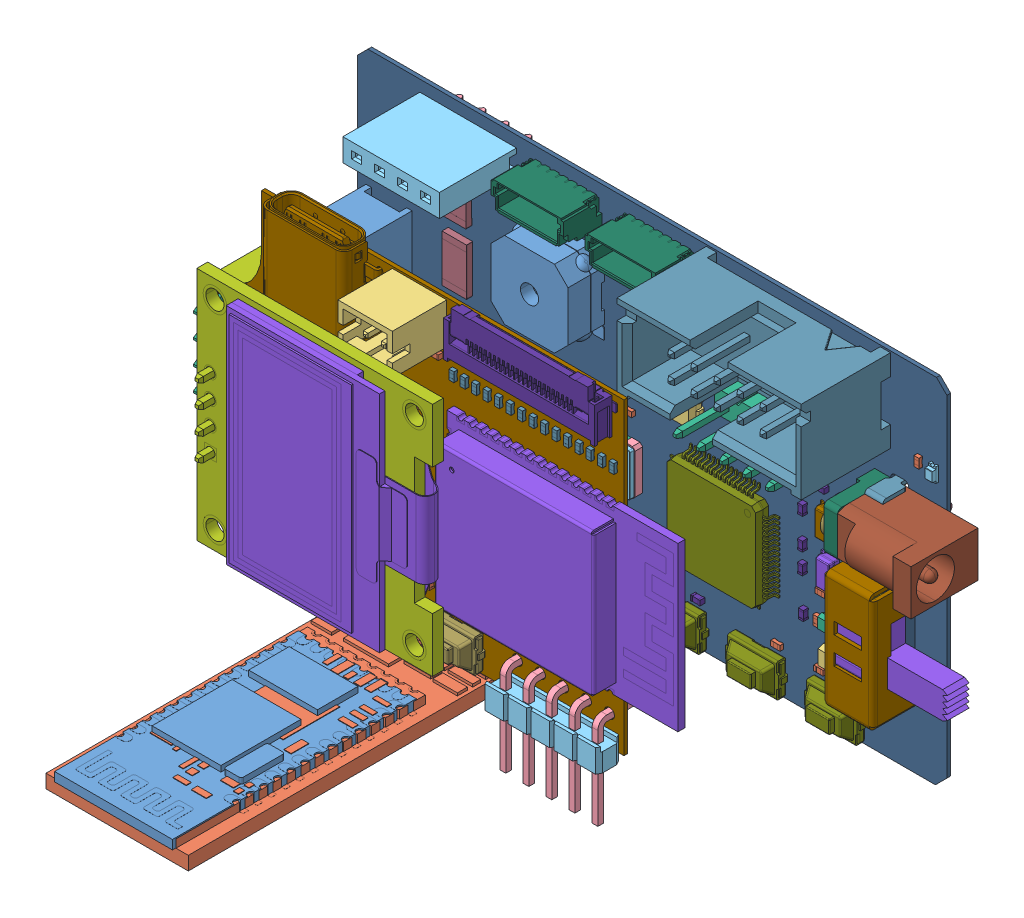
SolidWorks assembly balancing_robot_board, configuration Default. Lengths in mm.
Overall size (69.07 43.84 49.2).
373 component instances, 64 part files, 0 mates.
Components (placement in the parent):
- balancing_robot_board.step-1: balancing_robot_board.step [Default] at origin size (69.07 43.84 49.2)
  - LS.step-1: LS.step [Default] at origin size (8.5 8.5 4.05)
    - KSSG74B17-3--3DModel-STEP-532303.step-1: KSSG74B17-3--3DModel-STEP-532303.step [Default] at (18.4151 23.5629 3.048) x (0 1 0) z (1 0 0) size (8.5 4.05 8.5)
  - R23.step-1: R23.step [Default] at origin size (1.05 0.55 0.4)
    - RES_0402_(1005_metric).step-1: RES_0402_(1005_metric).step [Default] at (30.8864 22.1487 -0.4115) x (1 0 0) z (0 0 -1) size (1.05 0.55 0.4)
  - R21.step-1: R21.step [Default] at origin size (1.05 0.55 0.4)
    - RES_0402_(1005_metric).step-1: RES_0402_(1005_metric).step [Default] at (30.8864 25.3491 -0.4115) x (1 0 0) z (0 0 -1) size (1.05 0.55 0.4)
  - R22.step-1: R22.step [Default] at origin size (1.05 0.55 0.4)
    - RES_0402_(1005_metric).step-1: RES_0402_(1005_metric).step [Default] at (30.8864 23.7489 -0.4115) x (1 0 0) z (0 0 -1) size (1.05 0.55 0.4)
  - D5.step-1: D5.step [Default] at origin size (1.6 0.8 0.7)
    - 6715996480.step-1: 6715996480.step [Default] at (6.731 0.5588 0) x (1 0 0) z (0 -1 0) size (1.6 0.7 0.8)
  - D4.step-1: D4.step [Default] at origin size (1.6 0.8 0.7)
    - 6715996096.step-1: 6715996096.step [Default] at (46.7106 21.463 0) x (1 0 0) z (0 -1 0) size (1.6 0.7 0.8)
  - D3.step-1: D3.step [Default] at origin size (0.8 1.6 0.7)
    - 6715995904.step-1: 6715995904.step [Default] at (63.3476 29.1846 0) x (0 1 0) z (1 0 0) size (1.6 0.7 0.8)
  - Q1.step-1: Q1.step [Default] at origin size (2.92 2.37 1.12)
    - 6715995712.step-1: 6715995712.step [Default] at (52.8829 9.3981 0) x (0 1 0) z (1 0 0) size (2.37 1.12 2.92)
  - S1.step-1: S1.step [Default] at origin size (12.2 13 8.6)
    - User_Library-Assem1-20.step-1: User_Library-Assem1-20.step [Default] at (41.4801 49.8595 5.0375) x (0 1 0) z (1 0 0) size (13 8.6 12.2)
      - User_Library-Assem1-20_Part1.step-1: User_Library-Assem1-20_Part1.step [Default] at (-40.4363 -8.049 18.1299) size (1.5 6.6 0.5)
      - User_Library-Assem1-20_Part3.step-1: User_Library-Assem1-20_Part3.step [Default] at (-40.0863 -3.449 20.2299) size (9 3.9 11.7)
      - User_Library-Assem1-20_Part2.step-1: User_Library-Assem1-20_Part2.step [Default] at (-43.1863 0.551 15.4299) size (13 6 5.6)
      - User_Library-Assem1-20_Part1.step-2: User_Library-Assem1-20_Part1.step [Default] at (-37.4363 -8.049 18.1299) size (1.5 6.6 0.5)
      - User_Library-Assem1-20_Part1.step-3: User_Library-Assem1-20_Part1.step [Default] at (-34.4363 -8.049 18.1299) size (1.5 6.6 0.5)
      - User_Library-Assem1-20_Part4.step-1: User_Library-Assem1-20_Part4.step [Default] at (-30.9863 -4.449 15.5299) size (12.2 1 4.7)
  - ON_OFF.step-1: ON_OFF.step [Default] at origin size (11.6 5.4 10.6)
    - PJ-031D.step-1: PJ-031D.step [Default] at (68.0973 23.6729 0) x (0 1 0) z (1 0 0) size (5 7.4 9.5)
    - PJ-031D-0.step-1: PJ-031D-0.step [Default] at (68.0973 23.6729 0) x (0 1 0) z (1 0 0) size (3 9.2 0.6)
    - PJ-031D-1.step-1: PJ-031D-1.step [Default] at (68.0973 23.6729 0) x (0 1 0) z (1 0 0) size (1 3.2 0.3)
    - PJ-031D-2.step-1: PJ-031D-2.step [Default] at (68.0973 23.6729 0) x (0 1 0) z (1 0 0) size (0.4 6.2 2)
    - PJ-031D-3.step-1: PJ-031D-3.step [Default] at (68.0973 23.6729 0) x (0 1 0) z (1 0 0) size (5 6 1.9)
  - RESET.step-1: RESET.step [Default] at origin size (6.1 3.7 2.5)
    - User_Library-Button-SMD.step-1: User_Library-Button-SMD.step [Default] at (35.4637 1.3971 0) x (1 0 0) z (0 -1 0) size (6.1 2.5 3.7)
  - R14.step-1: R14.step [Default] at origin size (1.05 0.55 0.4)
    - RES_0402_(1005_metric).step-1: RES_0402_(1005_metric).step [Default] at (33.5534 4.1911 0) x (1 0 0) z (0 0 1) size (1.05 0.55 0.4)
  - C20.step-1: C20.step [Default] at origin size (1.05 0.55 0.55)
    - CAP_0402_(1005_metric).step-1: CAP_0402_(1005_metric).step [Default] at (37.4396 4.1909 0) x (-1 0 0) z (0 0 1) size (1.05 0.55 0.55)
  - C19.step-1: C19.step [Default] at origin size (5.08 10.66 11.6)
    - 61300821821.step-1: 61300821821.step [Default] at (3.1241 19.9389 4.26) x (0 1 0) z (0 0 1) size (10.66 5.08 11.6)
      - 6130xx21821_PIN.step-1: 6130xx21821_PIN.step [Default] at (-3.81 -1.47 -3.3268) size (2 0.4 10.2)
      - 6130xx21821_PIN.step-2: 6130xx21821_PIN.step [Default] at (-3.81 1.07 -3.3268) size (2 0.4 10.2)
      - 6130xx21821_PIN.step-3: 6130xx21821_PIN.step [Default] at (-1.27 -1.47 -3.3268) size (2 0.4 10.2)
      - 6130xx21821_PIN.step-4: 6130xx21821_PIN.step [Default] at (-1.27 1.07 -3.3268) size (2 0.4 10.2)
      - 6130xx21821_PIN.step-5: 6130xx21821_PIN.step [Default] at (1.27 -1.47 -3.3268) size (2 0.4 10.2)
      - 6130xx21821_PIN.step-6: 6130xx21821_PIN.step [Default] at (1.27 1.07 -3.3268) size (2 0.4 10.2)
      - 6130xx21821_PIN.step-7: 6130xx21821_PIN.step [Default] at (3.81 -1.47 -3.3268) size (2 0.4 10.2)
      - 6130xx21821_PIN.step-8: 6130xx21821_PIN.step [Default] at (3.81 1.07 -3.3268) size (2 0.4 10.2)
      - 61300821821-4.step-1: 61300821821-4.step [Default] at origin size (10.66 5.08 8.5)
  - STA.TR4.step-1: STA.TR4.step [Default] at origin size (1.4 3 1.14)
    - 6813825728.step-1: 6813825728.step [Default] at (25.1206 29.2354 -1.5515) size (1.4 3 1.14)
      - Extruded.step-1: Extruded.step [Default] at origin size (1.4 3 1.14)
  - STA.TR2.step-1: STA.TR2.step [Default] at origin size (1.4 3 1.14)
    - 6813825728.step-1: 6813825728.step [Default] at (29.9466 29.2354 -1.5515) size (1.4 3 1.14)
      - Extruded.step-1: Extruded.step [Default] at origin size (1.4 3 1.14)
  - STA.TR1.step-1: STA.TR1.step [Default] at origin size (1.4 3 1.14)
    - 6813825728.step-1: 6813825728.step [Default] at (34.798 29.2354 -1.5515) size (1.4 3 1.14)
      - Extruded.step-1: Extruded.step [Default] at origin size (1.4 3 1.14)
  - R28.step-1: R28.step [Default] at origin size (0.55 1.05 0.4)
    - RES_0402_(1005_metric).step-1: RES_0402_(1005_metric).step [Default] at (27.5589 29.6926 -0.4115) x (0 -1 0) z (0 0 -1) size (1.05 0.55 0.4)
  - R27.step-1: R27.step [Default] at origin size (0.55 1.05 0.4)
    - RES_0402_(1005_metric).step-1: RES_0402_(1005_metric).step [Default] at (32.3595 29.6926 -0.4115) x (0 -1 0) z (0 0 -1) size (1.05 0.55 0.4)
  - R24.step-1: R24.step [Default] at origin size (0.55 1.05 0.4)
    - RES_0402_(1005_metric).step-1: RES_0402_(1005_metric).step [Default] at (37.1855 29.6926 -0.4115) x (0 -1 0) z (0 0 -1) size (1.05 0.55 0.4)
  - R20.step-1: R20.step [Default] at origin size (1.05 0.55 0.4)
    - RES_0402_(1005_metric).step-1: RES_0402_(1005_metric).step [Default] at (46.1344 4.1401 0) x (-1 0 0) z (0 0 1) size (1.05 0.55 0.4)
  - R19.step-1: R19.step [Default] at origin size (1.05 0.55 0.4)
    - RES_0402_(1005_metric).step-1: RES_0402_(1005_metric).step [Default] at (50.8762 4.1403 0) x (1 0 0) z (0 0 1) size (1.05 0.55 0.4)
  - D2.step-1: D2.step [Default] at origin size (5.4 5 1.6)
    - 6715994176.step-1: 6715994176.step [Default] at (35.2806 23.749 0) x (1 0 0) z (0 -1 0) size (5.4 1.6 5)
  - CT1.step-1: CT1.step [Default] at origin size (3.2 5 1.3)
    - User_Library-ABM3-1.step-1: User_Library-ABM3-1.step [Default] at (29.5014 13.2335 0) x (0 1 0) z (0 0 1) size (5 3.2 1.3)
      - User_Library-ABM3-1_Fillet002.step-1: User_Library-ABM3-1_Fillet002.step [Default] at origin size (5 3.2 0.85)
      - User_Library-ABM3-1_Fillet001.step-1: User_Library-ABM3-1_Fillet001.step [Default] at (0 0 0.85) size (4.7 2.97 0.45)
      - User_Library-ABM3-1_Pad001.step-1: User_Library-ABM3-1_Pad001.step [Default] at origin size (4.9 2 0.4)
  - C18.step-1: C18.step [Default] at origin size (0.55 1.05 0.55)
    - CAP_0402_(1005_metric).step-1: CAP_0402_(1005_metric).step [Default] at (26.5297 10.9474 0) x (0 -1 0) z (0 0 1) size (1.05 0.55 0.55)
  - C17.step-1: C17.step [Default] at origin size (0.55 1.05 0.55)
    - CAP_0402_(1005_metric).step-1: CAP_0402_(1005_metric).step [Default] at (26.5295 15.494 0) x (0 1 0) z (0 0 1) size (1.05 0.55 0.55)
  - U5.step-1: U5.step [Default] at origin size (3 3 1.05)
    - 6715990144.step-1: 6715990144.step [Default] at (18.3896 16.1544 0) x (1 0 0) z (0 -1 0) size (3 1.05 3)
  - U4.step-1: U4.step [Default] at origin size (2.8 2.9 1.45)
    - 6715990912.step-1: 6715990912.step [Default] at (52.3494 14.4526 0) x (-1 0 0) z (0 1 0) size (2.8 1.45 2.9)
  - U3.step-1: U3.step [Default] at origin size (2.8 2.9 1.45)
    - 6715993792.step-1: 6715993792.step [Default] at (52.2478 19.1262 0) x (-1 0 0) z (0 1 0) size (2.8 1.45 2.9)
  - U2.step-1: U2.step [Default] at origin size (7 6.5 1.8)
    - 6715989760.step-1: 6715989760.step [Default] at (20.193 6.8072 0) x (1 0 0) z (0 -1 0) size (7 1.8 6.5)
  - U1.step-1: U1.step [Default] at origin size (3 3 1)
    - 6715991872.step-1: 6715991872.step [Default] at (4.8768 9.2964 0) x (-1 0 0) z (0 1 0) size (3 1 3)
  - SW2.step-1: SW2.step [Default] at origin size (6.1 3.7 2.5)
    - User_Library-Button-SMD.step-1: User_Library-Button-SMD.step [Default] at (44.1707 1.3971 0) x (1 0 0) z (0 -1 0) size (6.1 2.5 3.7)
  - SW1.step-1: SW1.step [Default] at origin size (6.1 3.7 2.5)
    - User_Library-Button-SMD.step-1: User_Library-Button-SMD.step [Default] at (52.8573 1.3969 0) x (-1 0 0) z (0 1 0) size (6.1 2.5 3.7)
  - STA.TR3.step-1: STA.TR3.step [Default] at origin size (1.4 3 1.14)
    - 6813825728.step-1: 6813825728.step [Default] at (19.7358 29.2354 -1.5515) size (1.4 3 1.14)
      - Extruded.step-1: Extruded.step [Default] at origin size (1.4 3 1.14)
  - R26.step-1: R26.step [Default] at origin size (0.55 1.05 0.4)
    - RES_0402_(1005_metric).step-1: RES_0402_(1005_metric).step [Default] at (22.5297 29.6926 -0.4115) x (0 -1 0) z (0 0 -1) size (1.05 0.55 0.4)
  - R25.step-1: R25.step [Default] at origin size (1.35 2.2 0.7)
    - RES_0805_(2012_metric).step-1: RES_0805_(2012_metric).step [Default] at (16.3323 24.5617 -0.013) x (0 -1 0) z (0 0 1) size (2.2 1.35 0.7)
  - R18.step-1: R18.step [Default] at origin size (0.55 1.05 0.4)
    - RES_0402_(1005_metric).step-1: RES_0402_(1005_metric).step [Default] at (61.6965 29.4466 0) x (0 1 0) z (0 0 1) size (1.05 0.55 0.4)
  - R17.step-1: R17.step [Default] at origin size (0.55 1.05 0.4)
    - RES_0402_(1005_metric).step-1: RES_0402_(1005_metric).step [Default] at (9.2455 0.5588 0) x (0 1 0) z (0 0 1) size (1.05 0.55 0.4)
  - R16.step-1: R16.step [Default] at origin size (0.55 1.05 0.4)
    - RES_0402_(1005_metric).step-1: RES_0402_(1005_metric).step [Default] at (48.9965 21.0646 0) x (0 1 0) z (0 0 1) size (1.05 0.55 0.4)
  - R15.step-1: R15.step [Default] at origin size (1.05 0.55 0.4)
    - RES_0402_(1005_metric).step-1: RES_0402_(1005_metric).step [Default] at (29.7608 18.2625 0) x (-1 0 0) z (0 0 1) size (1.05 0.55 0.4)
  - R13.step-1: R13.step [Default] at origin size (0.55 1.05 0.4)
    - RES_0402_(1005_metric).step-1: RES_0402_(1005_metric).step [Default] at (1.2315 7.8282 0) x (0 1 0) z (0 0 1) size (1.05 0.55 0.4)
  - R12.step-1: R12.step [Default] at origin size (0.55 1.05 0.4)
    - RES_0402_(1005_metric).step-1: RES_0402_(1005_metric).step [Default] at (1.2823 10.3094 0) x (0 1 0) z (0 0 1) size (1.05 0.55 0.4)
  - R11.step-1: R11.step [Default] at origin size (1.05 0.55 0.4)
    - RES_0402_(1005_metric).step-1: RES_0402_(1005_metric).step [Default] at (1.7316 5.5087 0) x (-1 0 0) z (0 0 1) size (1.05 0.55 0.4)
  - R10.step-1: R10.step [Default] at origin size (1.05 0.55 0.4)
    - RES_0402_(1005_metric).step-1: RES_0402_(1005_metric).step [Default] at (5.8544 12.8495 0) x (1 0 0) z (0 0 1) size (1.05 0.55 0.4)
  - R9.step-1: R9.step [Default] at origin size (0.55 1.05 0.4)
    - RES_0402_(1005_metric).step-1: RES_0402_(1005_metric).step [Default] at (8.2927 8.0742 0) x (0 1 0) z (0 0 1) size (1.05 0.55 0.4)
  - R8.step-1: R8.step [Default] at origin size (0.55 1.05 0.4)
    - RES_0402_(1005_metric).step-1: RES_0402_(1005_metric).step [Default] at (8.2675 10.4364 0) x (0 -1 0) z (0 0 1) size (1.05 0.55 0.4)
  - R7.step-1: R7.step [Default] at origin size (2.7 5.2 0.7)
    - RES_2010_(5025_metric).step-1: RES_2010_(5025_metric).step [Default] at (10.9221 29.7687 -0.013) x (0 -1 0) z (0 0 1) size (5.2 2.7 0.7)
  - R6.step-1: R6.step [Default] at origin size (2.7 5.2 0.7)
    - RES_2010_(5025_metric).step-1: RES_2010_(5025_metric).step [Default] at (10.9981 23.0773 -0.013) x (0 1 0) z (0 0 1) size (5.2 2.7 0.7)
  - R5.step-1: R5.step [Default] at origin size (0.55 1.05 0.4)
    - RES_0402_(1005_metric).step-1: RES_0402_(1005_metric).step [Default] at (13.8939 7.239 0) x (0 -1 0) z (0 0 1) size (1.05 0.55 0.4)
  - R4.step-1: R4.step [Default] at origin size (0.55 1.05 0.4)
    - RES_0402_(1005_metric).step-1: RES_0402_(1005_metric).step [Default] at (13.8939 4.9276 0) x (0 -1 0) z (0 0 1) size (1.05 0.55 0.4)
  - R3.step-1: R3.step [Default] at origin size (1.05 0.55 0.4)
    - RES_0402_(1005_metric).step-1: RES_0402_(1005_metric).step [Default] at (51.0286 11.6333 0) x (1 0 0) z (0 0 1) size (1.05 0.55 0.4)
  - R2.step-1: R2.step [Default] at origin size (1.05 0.55 0.4)
    - RES_0402_(1005_metric).step-1: RES_0402_(1005_metric).step [Default] at (54.8386 11.6333 0) x (1 0 0) z (0 0 1) size (1.05 0.55 0.4)
  - R1.step-1: R1.step [Default] at origin size (0.55 1.05 0.4)
    - RES_0402_(1005_metric).step-1: RES_0402_(1005_metric).step [Default] at (50.5461 8.6948 0) x (0 -1 0) z (0 0 1) size (1.05 0.55 0.4)
  - P1.step-1: P1.step [Default] at origin size (20.32 9.14 12.9)
    - User_Library-Tyco_-_5103308-1_(Shrouded_Header_2_54mm_10_Pin).step-1: User_Library-Tyco_-_5103308-1_(Shrouded_Header_2_54mm_10_Pin).step [Default] at (48.2856 33.5278 0) x (1 0 0) z (0 -1 0) size (20.32 12.9 9.14)
  - J4.step-1: J4.step [Default] at origin size (8 3.6 4.25)
    - 6715990528.step-1: 6715990528.step [Default] at (22.606 36.2966 0) x (1 0 0) z (0 -1 0) size (8 4.25 3.6)
      - BMxxB-SRSS-TB(LF)(SN)_06.step-1: BMxxB-SRSS-TB(LF)(SN)_06.step [Default] at (0 0 0.75) size (8 4.25 3.6)
  - J3.step-1: J3.step [Default] at origin size (8 3.6 4.25)
    - 6715990528.step-1: 6715990528.step [Default] at (32.9932 36.2682 0) x (1 0 0) z (0 -1 0) size (8 4.25 3.6)
      - BMxxB-SRSS-TB(LF)(SN)_06.step-1: BMxxB-SRSS-TB(LF)(SN)_06.step [Default] at (0 0 0.75) size (8 4.25 3.6)
  - J1.step-1: J1.step [Default] at origin size (12 12 1.6)
    - 6715993024.step-1: 6715993024.step [Default] at (40.259 12.4714 0) x (0 -1 0) z (-1 0 0) size (12 1.6 12)
  - HC1.step-1: HC1.step [Default] at origin size (15.74 7.73 49.09)
    - 61300611821.step-1: 61300611821.step [Default] at (18.7197 0.9143 4.26) x (-1 0 0) z (0 0 1) size (15.74 2.5 11.6)
      - 6130xx11821_PIN.step-1: 6130xx11821_PIN.step [Default] at (-6.35 -0.2 -3.3268) size (2 0.4 10.2)
      - 6130xx11821_PIN.step-2: 6130xx11821_PIN.step [Default] at (-3.81 -0.2 -3.3268) size (2 0.4 10.2)
      - 6130xx11821_PIN.step-3: 6130xx11821_PIN.step [Default] at (-1.27 -0.2 -3.3268) size (2 0.4 10.2)
      - 6130xx11821_PIN.step-4: 6130xx11821_PIN.step [Default] at (1.27 -0.2 -3.3268) size (2 0.4 10.2)
      - 6130xx11821_PIN.step-5: 6130xx11821_PIN.step [Default] at (3.81 -0.2 -3.3268) size (2 0.4 10.2)
      - 6130xx11821_PIN.step-6: 6130xx11821_PIN.step [Default] at (6.35 -0.2 -3.3268) size (2 0.4 10.2)
      - 61300611821-5.step-1: 61300611821-5.step [Default] at origin size (15.74 2.5 8.5)
    - HC-06.step-1: HC-06.step [Default] at (25.2198 -3.0227 46) x (0 0 -1) z (1 0 0) size (26.9 1.63 13)
    - Bluetooth_4.0_BLE.step-1: Bluetooth_4.0_BLE.step [Default] at (18.7199 -3.0627 8) x (0 0 1) z (-1 0 0) size (44.38 6.8 15.7)
  - D1.step-1: D1.step [Default] at origin size (3.9 1.8 1.18)
    - SOD123.step-1: SOD123.step [Default] at (52.9335 6.1975 0) x (-1 0 0) z (0 0 1) size (3.9 1.8 1.18)
  - C16.step-1: C16.step [Default] at origin size (10.66 2.5 11.6)
    - 61300411821.step-1: 61300411821.step [Default] at (11.8617 35.7885 4.26) x (-1 0 0) z (0 0 1) size (10.66 2.5 11.6)
      - 6130xx11821_PIN-6.step-1: 6130xx11821_PIN-6.step [Default] at (-3.81 -0.2 -3.3268) size (2 0.4 10.2)
      - 6130xx11821_PIN-6.step-2: 6130xx11821_PIN-6.step [Default] at (-1.27 -0.2 -3.3268) size (2 0.4 10.2)
      - 6130xx11821_PIN-6.step-3: 6130xx11821_PIN-6.step [Default] at (1.27 -0.2 -3.3268) size (2 0.4 10.2)
      - 6130xx11821_PIN-6.step-4: 6130xx11821_PIN-6.step [Default] at (3.81 -0.2 -3.3268) size (2 0.4 10.2)
      - 61300411821-7.step-1: 61300411821-7.step [Default] at origin size (10.66 2.5 8.5)
  - C15.step-1: C15.step [Default] at origin size (1.05 0.55 0.55)
    - CAP_0402_(1005_metric).step-1: CAP_0402_(1005_metric).step [Default] at (5.9306 5.5087 0) x (-1 0 0) z (0 0 1) size (1.05 0.55 0.55)
  - C14.step-1: C14.step [Default] at origin size (1.05 0.55 0.55)
    - CAP_0402_(1005_metric).step-1: CAP_0402_(1005_metric).step [Default] at (1.7956 12.8495 0) x (1 0 0) z (0 0 1) size (1.05 0.55 0.55)
  - C13.step-1: C13.step [Default] at origin size (0.55 1.05 0.55)
    - CAP_0402_(1005_metric).step-1: CAP_0402_(1005_metric).step [Default] at (9.8421 10.4284 0) x (0 1 0) z (0 0 1) size (1.05 0.55 0.55)
  - C12.step-1: C12.step [Default] at origin size (1.05 0.55 0.55)
    - CAP_0402_(1005_metric).step-1: CAP_0402_(1005_metric).step [Default] at (51.1302 21.6915 0) x (-1 0 0) z (0 0 1) size (1.05 0.55 0.55)
  - C11.step-1: C11.step [Default] at origin size (1.05 0.55 0.55)
    - CAP_0402_(1005_metric).step-1: CAP_0402_(1005_metric).step [Default] at (53.3734 21.6917 0) x (1 0 0) z (0 0 1) size (1.05 0.55 0.55)
  - C10.step-1: C10.step [Default] at origin size (0.55 1.05 0.55)
    - CAP_0402_(1005_metric).step-1: CAP_0402_(1005_metric).step [Default] at (49.0221 18.669 0) x (0 -1 0) z (0 0 1) size (1.05 0.55 0.55)
  - C9.step-1: C9.step [Default] at origin size (1.05 0.55 0.55)
    - CAP_0402_(1005_metric).step-1: CAP_0402_(1005_metric).step [Default] at (14.3938 9.2711 0) size (1.05 0.55 0.55)
  - C8.step-1: C8.step [Default] at origin size (0.55 1.05 0.55)
    - CAP_0402_(1005_metric).step-1: CAP_0402_(1005_metric).step [Default] at (19.9899 12.4968 0) x (0 -1 0) z (0 0 1) size (1.05 0.55 0.55)
  - C7.step-1: C7.step [Default] at origin size (1.05 0.55 0.55)
    - CAP_0402_(1005_metric).step-1: CAP_0402_(1005_metric).step [Default] at (17.3482 11.7989 0) x (-1 0 0) z (0 0 1) size (1.05 0.55 0.55)
  - C6.step-1: C6.step [Default] at origin size (1.05 0.55 0.55)
    - CAP_0402_(1005_metric).step-1: CAP_0402_(1005_metric).step [Default] at (17.3176 13.0555 0) x (-1 0 0) z (0 0 1) size (1.05 0.55 0.55)
  - C5.step-1: C5.step [Default] at origin size (0.55 1.05 0.55)
    - CAP_0402_(1005_metric).step-1: CAP_0402_(1005_metric).step [Default] at (48.9965 12.9794 0) x (0 1 0) z (0 0 1) size (1.05 0.55 0.55)
  - C4.step-1: C4.step [Default] at origin size (0.55 1.05 0.55)
    - CAP_0402_(1005_metric).step-1: CAP_0402_(1005_metric).step [Default] at (48.9967 15.24 0) x (0 -1 0) z (0 0 1) size (1.05 0.55 0.55)
  - C3.step-1: C3.step [Default] at origin size (0.55 1.05 0.55)
    - CAP_0402_(1005_metric).step-1: CAP_0402_(1005_metric).step [Default] at (55.1943 14.9098 0) x (0 -1 0) z (0 0 1) size (1.05 0.55 0.55)
  - C2.step-1: C2.step [Default] at origin size (0.55 1.05 0.55)
    - CAP_0402_(1005_metric).step-1: CAP_0402_(1005_metric).step [Default] at (49.0981 8.6614 0) x (0 1 0) z (0 0 1) size (1.05 0.55 0.55)
  - C1.step-1: C1.step [Default] at origin size (0.55 1.05 0.55)
    - CAP_0402_(1005_metric).step-1: CAP_0402_(1005_metric).step [Default] at (55.2703 8.6948 0) x (0 1 0) z (0 0 1) size (1.05 0.55 0.55)
  - _.step-1: _.step [Default] at origin size (12.6 2.5 11.2)
    - JP1-5.step-1: JP1-5.step [Default] at (47.9289 26.4613 0.0152) x (1 0 0) z (0 1 0) size (12.6 11.2 2.5)
  - Free-Models.step-1: Free-Models.step [Default] at origin size (52.76 42.29 17.88)
    - ESP32_DEV1.step-1: ESP32_DEV1.step [Default] at (6.534 2.6352 17.5) size (52.76 42.29 17.88)
      - U.step-1: U.step [Default] at origin size (26 26 11.3)
        - 16300172544.step-1: 16300172544.step [Default] at (13.335 17.2212 3.302) x (0 1 0) z (1 0 0) size (26 11.3 26)
          - DM-OLED096-636_Module.step-1: DM-OLED096-636_Module.step [Default] at origin size (26 11.3 26)
          - DM-OLED096-636_Panel.step-1: DM-OLED096-636_Panel.step [Default] at (0 4.16 0) size (24.74 2.81 21.35)
      - USB.step-1: USB.step [Default] at origin size (11.9 10.14 3.89)
        - 18613833344.step-1: 18613833344.step [Default] at (7.2528 35.2469 1.0668) x (-1 0 0) z (0 1 0) size (11.9 3.89 10.14)
      - U3-1.step-1: U3-1.step [Default] at origin size (3 3 0.9)
        - 17995934848.step-1: 17995934848.step [Default] at (15.8202 15.8114 0) x (1 0 0) z (0 -1 0) size (3 0.9 3)
      - U1-1.step-1: U1-1.step [Default] at origin size (6.5 7 1.8)
        - 15937648576.step-1: 15937648576.step [Default] at (3.5598 4.0213 0) x (-1 0 0) z (0 1 0) size (6.5 1.8 7)
      - SW2-1.step-1: SW2-1.step [Default] at origin size (6.1 3.7 2.5)
        - User_Library-Button-SMD-8.step-1: User_Library-Button-SMD-8.step [Default] at (21.7423 1.9049 0) x (-1 0 0) z (0 1 0) size (6.1 2.5 3.7)
      - SW1-1.step-1: SW1-1.step [Default] at origin size (6.1 3.7 2.5)
        - User_Library-Button-SMD-8.step-1: User_Library-Button-SMD-8.step [Default] at (12.9539 1.9049 0) x (-1 0 0) z (0 1 0) size (6.1 2.5 3.7)
      - STA.TR2-1.step-1: STA.TR2-1.step [Default] at origin size (3 1.4 1.14)
        - 7019244480.step-1: 7019244480.step [Default] at (36.6522 9.9904 -1.5413) size (3 1.4 1.14)
          - Extruded-9.step-1: Extruded-9.step [Default] at origin size (3 1.4 1.14)
      - STA.TR1-1.step-1: STA.TR1-1.step [Default] at origin size (3 1.4 1.14)
        - 7019244480.step-1: 7019244480.step [Default] at (29.9212 10.0045 -1.5413) size (3 1.4 1.14)
          - Extruded-9.step-1: Extruded-9.step [Default] at origin size (3 1.4 1.14)
      - R30.step-1: R30.step [Default] at origin size (0.55 1.05 0.4)
        - RES_0402_(1005_metric)-10.step-1: RES_0402_(1005_metric)-10.step [Default] at (15.2735 12.2508 0) x (0 -1 0) z (0 0 1) size (1.05 0.55 0.4)
      - R29.step-1: R29.step [Default] at origin size (0.55 1.05 0.4)
        - RES_0402_(1005_metric)-10.step-1: RES_0402_(1005_metric)-10.step [Default] at (14.0289 12.2508 0) x (0 -1 0) z (0 0 1) size (1.05 0.55 0.4)
      - R28-1.step-1: R28-1.step [Default] at origin size (0.55 1.05 0.4)
        - RES_0402_(1005_metric)-10.step-1: RES_0402_(1005_metric)-10.step [Default] at (10.2109 22.2706 0) x (0 -1 0) z (0 0 1) size (1.05 0.55 0.4)
      - R27-1.step-1: R27-1.step [Default] at origin size (0.55 1.05 0.4)
        - RES_0402_(1005_metric)-10.step-1: RES_0402_(1005_metric)-10.step [Default] at (8.8899 22.2706 0) x (0 1 0) z (0 0 1) size (1.05 0.55 0.4)
      - R26-1.step-1: R26-1.step [Default] at origin size (0.55 1.05 0.4)
        - RES_0402_(1005_metric)-10.step-1: RES_0402_(1005_metric)-10.step [Default] at (14.8591 22.225 0) x (0 -1 0) z (0 0 1) size (1.05 0.55 0.4)
      - R25-1.step-1: R25-1.step [Default] at origin size (0.55 1.05 0.4)
        - RES_0402_(1005_metric)-10.step-1: RES_0402_(1005_metric)-10.step [Default] at (14.8845 19.812 0) x (0 -1 0) z (0 0 1) size (1.05 0.55 0.4)
      - R24-1.step-1: R24-1.step [Default] at origin size (0.55 1.05 0.4)
        - RES_0402_(1005_metric)-10.step-1: RES_0402_(1005_metric)-10.step [Default] at (37.7699 26.9748 0) x (0 -1 0) z (0 0 1) size (1.05 0.55 0.4)
      - R23-1.step-1: R23-1.step [Default] at origin size (0.55 1.05 0.4)
        - RES_0402_(1005_metric)-10.step-1: RES_0402_(1005_metric)-10.step [Default] at (39.0145 26.9748 0) x (0 -1 0) z (0 0 1) size (1.05 0.55 0.4)
      - R22-1.step-1: R22-1.step [Default] at origin size (1.05 0.55 0.4)
        - RES_0402_(1005_metric)-10.step-1: RES_0402_(1005_metric)-10.step [Default] at (21.717 3.0479 -0.4013) x (1 0 0) z (0 0 -1) size (1.05 0.55 0.4)
      - R21-1.step-1: R21-1.step [Default] at origin size (1.05 0.55 0.4)
        - RES_0402_(1005_metric)-10.step-1: RES_0402_(1005_metric)-10.step [Default] at (35.814 32.6135 -0.4013) x (1 0 0) z (0 0 -1) size (1.05 0.55 0.4)
      - R20-1.step-1: R20-1.step [Default] at origin size (1.05 0.55 0.4)
        - RES_0402_(1005_metric)-10.step-1: RES_0402_(1005_metric)-10.step [Default] at (13.0048 3.2511 -0.4115) x (1 0 0) z (0 0 -1) size (1.05 0.55 0.4)
      - R19-1.step-1: R19-1.step [Default] at origin size (0.55 1.05 0.4)
        - RES_0402_(1005_metric)-10.step-1: RES_0402_(1005_metric)-10.step [Default] at (36.4997 26.9748 0) x (0 1 0) z (0 0 1) size (1.05 0.55 0.4)
      - R18-1.step-1: R18-1.step [Default] at origin size (0.55 1.05 0.4)
        - RES_0402_(1005_metric)-10.step-1: RES_0402_(1005_metric)-10.step [Default] at (35.2551 26.9748 0) x (0 1 0) z (0 0 1) size (1.05 0.55 0.4)
      - R17-1.step-1: R17-1.step [Default] at origin size (0.55 1.05 0.4)
        - RES_0402_(1005_metric)-10.step-1: RES_0402_(1005_metric)-10.step [Default] at (33.9851 26.9748 0) x (0 1 0) z (0 0 1) size (1.05 0.55 0.4)
      - R16-1.step-1: R16-1.step [Default] at origin size (0.55 1.05 0.4)
        - RES_0402_(1005_metric)-10.step-1: RES_0402_(1005_metric)-10.step [Default] at (38.9889 10.541 -0.4013) x (0 -1 0) z (0 0 -1) size (1.05 0.55 0.4)
      - R15-1.step-1: R15-1.step [Default] at origin size (0.55 1.05 0.4)
        - RES_0402_(1005_metric)-10.step-1: RES_0402_(1005_metric)-10.step [Default] at (32.7151 26.9494 0) x (0 1 0) z (0 0 1) size (1.05 0.55 0.4)
      - R14-1.step-1: R14-1.step [Default] at origin size (0.55 1.05 0.4)
        - RES_0402_(1005_metric)-10.step-1: RES_0402_(1005_metric)-10.step [Default] at (34.3153 10.5156 -0.4013) x (0 -1 0) z (0 0 -1) size (1.05 0.55 0.4)
      - R13-1.step-1: R13-1.step [Default] at origin size (0.55 1.05 0.4)
        - RES_0402_(1005_metric)-10.step-1: RES_0402_(1005_metric)-10.step [Default] at (31.4451 26.9494 0) x (0 1 0) z (0 0 1) size (1.05 0.55 0.4)
      - R12-1.step-1: R12-1.step [Default] at origin size (0.55 1.05 0.4)
        - RES_0402_(1005_metric)-10.step-1: RES_0402_(1005_metric)-10.step [Default] at (30.2005 26.9494 0) x (0 1 0) z (0 0 1) size (1.05 0.55 0.4)
      - R11-1.step-1: R11-1.step [Default] at origin size (0.55 1.05 0.4)
        - RES_0402_(1005_metric)-10.step-1: RES_0402_(1005_metric)-10.step [Default] at (28.9305 26.9494 0) x (0 1 0) z (0 0 1) size (1.05 0.55 0.4)
      - R10-1.step-1: R10-1.step [Default] at origin size (0.55 1.05 0.4)
        - RES_0402_(1005_metric)-10.step-1: RES_0402_(1005_metric)-10.step [Default] at (27.6605 26.9494 0) x (0 1 0) z (0 0 1) size (1.05 0.55 0.4)
      - R9-1.step-1: R9-1.step [Default] at origin size (0.55 1.05 0.4)
        - RES_0402_(1005_metric)-10.step-1: RES_0402_(1005_metric)-10.step [Default] at (26.3905 26.9494 0) x (0 1 0) z (0 0 1) size (1.05 0.55 0.4)
      - R8-1.step-1: R8-1.step [Default] at origin size (0.55 1.05 0.4)
        - RES_0402_(1005_metric)-10.step-1: RES_0402_(1005_metric)-10.step [Default] at (27.6097 10.541 -0.4013) x (0 -1 0) z (0 0 -1) size (1.05 0.55 0.4)
      - R7-1.step-1: R7-1.step [Default] at origin size (0.55 1.05 0.4)
        - RES_0402_(1005_metric)-10.step-1: RES_0402_(1005_metric)-10.step [Default] at (25.1205 26.924 0) x (0 1 0) z (0 0 1) size (1.05 0.55 0.4)
      - R6-1.step-1: R6-1.step [Default] at origin size (0.55 1.05 0.4)
        - RES_0402_(1005_metric)-10.step-1: RES_0402_(1005_metric)-10.step [Default] at (23.8505 26.924 0) x (0 1 0) z (0 0 1) size (1.05 0.55 0.4)
      - R5-1.step-1: R5-1.step [Default] at origin size (0.55 1.05 0.4)
        - RES_0402_(1005_metric)-10.step-1: RES_0402_(1005_metric)-10.step [Default] at (32.2325 10.541 -0.4013) x (0 -1 0) z (0 0 -1) size (1.05 0.55 0.4)
      - R4-1.step-1: R4-1.step [Default] at origin size (0.55 1.05 0.4)
        - RES_0402_(1005_metric)-10.step-1: RES_0402_(1005_metric)-10.step [Default] at (22.6059 26.924 0) x (0 1 0) z (0 0 1) size (1.05 0.55 0.4)
      - R3-1.step-1: R3-1.step [Default] at origin size (0.55 1.05 0.4)
        - RES_0402_(1005_metric)-10.step-1: RES_0402_(1005_metric)-10.step [Default] at (21.3613 26.924 0) x (0 1 0) z (0 0 1) size (1.05 0.55 0.4)
      - R2-1.step-1: R2-1.step [Default] at origin size (1.05 0.55 0.4)
        - RES_0402_(1005_metric)-10.step-1: RES_0402_(1005_metric)-10.step [Default] at (15.3416 24.9173 0) x (-1 0 0) z (0 0 1) size (1.05 0.55 0.4)
      - R1-1.step-1: R1-1.step [Default] at origin size (1.05 0.55 0.4)
        - RES_0402_(1005_metric)-10.step-1: RES_0402_(1005_metric)-10.step [Default] at (15.3416 26.1873 0) x (-1 0 0) z (0 0 1) size (1.05 0.55 0.4)
      - MK1.step-1: MK1.step [Default] at origin size (3.76 4.72 1.05)
        - 11871186624.step-1: 11871186624.step [Default] at (8.986 14.3002 0) x (0 -1 0) z (-1 0 0) size (4.72 1.05 3.76)
      - J4-1.step-1: J4-1.step [Default] at origin size (2.9 2.8 1.3)
        - 16119298752.step-1: 16119298752.step [Default] at (15.1386 6.477 0) x (0 -1 0) z (-1 0 0) size (2.8 1.3 2.9)
      - J3-1.step-1: J3-1.step [Default] at origin size (2.9 2.8 1.3)
        - 16119298752.step-1: 16119298752.step [Default] at (8.6616 6.477 0) x (0 -1 0) z (-1 0 0) size (2.8 1.3 2.9)
      - J2.step-1: J2.step [Default] at origin size (17.5 5.3 2.1)
        - 5051102491--3DModel-STEP-510211.step-1: 5051102491--3DModel-STEP-510211.step [Default] at (30.5147 32.6128 0) x (-1 0 0) z (0 1 0) size (17.5 2.1 5.3)
          - 5051102491_5051102491.step-1: 5051102491_5051102491.step [Default] at (0 0 -0.25) size (17.5 2.1 5.3)
      - D3-1.step-1: D3-1.step [Default] at origin size (0.8 1.6 0.7)
        - 19165414592.step-1: 19165414592.step [Default] at (5.6134 22.1234 0) x (0 1 0) z (1 0 0) size (1.6 0.7 0.8)
      - D2-1.step-1: D2-1.step [Default] at origin size (0.8 1.6 0.7)
        - 16293771392.step-1: 16293771392.step [Default] at (7.0612 22.1488 0) x (0 -1 0) z (-1 0 0) size (1.6 0.7 0.8)
      - D1-1.step-1: D1-1.step [Default] at origin size (0.8 1.6 0.7)
        - 19165414592.step-1: 19165414592.step [Default] at (4.1656 22.1488 0) x (0 1 0) z (1 0 0) size (1.6 0.7 0.8)
      - C31.step-1: C31.step [Default] at origin size (1.05 0.55 0.55)
        - CAP_0402_(1005_metric)-11.step-1: CAP_0402_(1005_metric)-11.step [Default] at (17.2038 11.6841 0) x (1 0 0) z (0 0 1) size (1.05 0.55 0.55)
      - C30.step-1: C30.step [Default] at origin size (1.05 0.55 0.55)
        - CAP_0402_(1005_metric)-11.step-1: CAP_0402_(1005_metric)-11.step [Default] at (17.1864 12.8525 0) x (1 0 0) z (0 0 1) size (1.05 0.55 0.55)
      - C29.step-1: C29.step [Default] at origin size (1.05 0.55 0.55)
        - CAP_0402_(1005_metric)-11.step-1: CAP_0402_(1005_metric)-11.step [Default] at (19.5326 28.0671 0) x (1 0 0) z (0 0 1) size (1.05 0.55 0.55)
      - C28.step-1: C28.step [Default] at origin size (1.05 0.55 0.55)
        - CAP_0402_(1005_metric)-11.step-1: CAP_0402_(1005_metric)-11.step [Default] at (15.367 28.0669 0) x (-1 0 0) z (0 0 1) size (1.05 0.55 0.55)
      - C27.step-1: C27.step [Default] at origin size (1.05 0.55 0.55)
        - CAP_0402_(1005_metric)-11.step-1: CAP_0402_(1005_metric)-11.step [Default] at (5.4102 12.4461 0) x (1 0 0) z (0 0 1) size (1.05 0.55 0.55)
      - C26.step-1: C26.step [Default] at origin size (1.05 0.55 0.55)
        - CAP_0402_(1005_metric)-11.step-1: CAP_0402_(1005_metric)-11.step [Default] at (5.4102 15.5957 0) x (1 0 0) z (0 0 1) size (1.05 0.55 0.55)
      - C25.step-1: C25.step [Default] at origin size (6 4.5 7.91)
        - User_Library-PCB_HEADER_(JST_BxB-PH-K-S_(VERTICAL)).step-1: User_Library-PCB_HEADER_(JST_BxB-PH-K-S_(VERTICAL)).step [Default] at (17.4498 31.2822 0) x (1 0 0) z (0 -1 0) size (6 7.91 4.5)
      - C24.step-1: C24.step [Default] at origin size (0.55 1.05 0.55)
        - CAP_0402_(1005_metric)-11.step-1: CAP_0402_(1005_metric)-11.step [Default] at (11.4555 22.2706 0) x (0 -1 0) z (0 0 1) size (1.05 0.55 0.55)
      - C22.step-1: C22.step [Default] at origin size (0.55 1.05 0.55)
        - CAP_0402_(1005_metric)-11.step-1: CAP_0402_(1005_metric)-11.step [Default] at (17.2465 22.225 0) x (0 1 0) z (0 0 1) size (1.05 0.55 0.55)
      - C21.step-1: C21.step [Default] at origin size (0.55 1.05 0.55)
        - CAP_0402_(1005_metric)-11.step-1: CAP_0402_(1005_metric)-11.step [Default] at (16.0781 22.225 0) x (0 1 0) z (0 0 1) size (1.05 0.55 0.55)
      - C20-1.step-1: C20-1.step [Default] at origin size (0.55 1.05 0.55)
        - CAP_0402_(1005_metric)-11.step-1: CAP_0402_(1005_metric)-11.step [Default] at (18.8215 5.8848 0) x (0 -1 0) z (0 0 1) size (1.05 0.55 0.55)
      - C19-1.step-1: C19-1.step [Default] at origin size (0.55 1.05 0.55)
        - CAP_0402_(1005_metric)-11.step-1: CAP_0402_(1005_metric)-11.step [Default] at (17.6785 5.8928 0) x (0 -1 0) z (0 0 1) size (1.05 0.55 0.55)
      - C18-1.step-1: C18-1.step [Default] at origin size (1.05 0.55 0.55)
        - CAP_0402_(1005_metric)-11.step-1: CAP_0402_(1005_metric)-11.step [Default] at (14.732 9.1439 0) x (-1 0 0) z (0 0 1) size (1.05 0.55 0.55)
      - C17-1.step-1: C17-1.step [Default] at origin size (1.05 0.55 0.55)
        - CAP_0402_(1005_metric)-11.step-1: CAP_0402_(1005_metric)-11.step [Default] at (18.2118 7.8231 0) x (-1 0 0) z (0 0 1) size (1.05 0.55 0.55)
      - C16-1.step-1: C16-1.step [Default] at origin size (1.05 0.55 0.55)
        - CAP_0402_(1005_metric)-11.step-1: CAP_0402_(1005_metric)-11.step [Default] at (8.2804 9.1439 0) x (-1 0 0) z (0 0 1) size (1.05 0.55 0.55)
      - C15-1.step-1: C15-1.step [Default] at origin size (1.05 0.55 0.55)
        - CAP_0402_(1005_metric)-11.step-1: CAP_0402_(1005_metric)-11.step [Default] at (11.6332 7.7977 0) x (-1 0 0) z (0 0 1) size (1.05 0.55 0.55)
      - C14-1.step-1: C14-1.step [Default] at origin size (0.55 1.05 0.55)
        - CAP_0402_(1005_metric)-11.step-1: CAP_0402_(1005_metric)-11.step [Default] at (17.2719 19.8374 0) x (0 1 0) z (0 0 1) size (1.05 0.55 0.55)
      - C13-1.step-1: C13-1.step [Default] at origin size (0.55 1.05 0.55)
        - CAP_0402_(1005_metric)-11.step-1: CAP_0402_(1005_metric)-11.step [Default] at (16.1289 19.8374 0) x (0 1 0) z (0 0 1) size (1.05 0.55 0.55)
      - C12-1.step-1: C12-1.step [Default] at origin size (0.55 1.05 0.55)
        - CAP_0402_(1005_metric)-11.step-1: CAP_0402_(1005_metric)-11.step [Default] at (11.0411 5.8928 0) x (0 -1 0) z (0 0 1) size (1.05 0.55 0.55)
      - C11-1.step-1: C11-1.step [Default] at origin size (0.55 1.05 0.55)
        - CAP_0402_(1005_metric)-11.step-1: CAP_0402_(1005_metric)-11.step [Default] at (12.2349 5.8928 0) x (0 -1 0) z (0 0 1) size (1.05 0.55 0.55)
      - C10-1.step-1: C10-1.step [Default] at origin size (1.05 0.55 0.55)
        - CAP_0402_(1005_metric)-11.step-1: CAP_0402_(1005_metric)-11.step [Default] at (4.072 10.2869 0) x (-1 0 0) z (0 0 1) size (1.05 0.55 0.55)
      - C9-1.step-1: C9-1.step [Default] at origin size (1.05 0.55 0.55)
        - CAP_0402_(1005_metric)-11.step-1: CAP_0402_(1005_metric)-11.step [Default] at (4.072 9.0169 0) x (-1 0 0) z (0 0 1) size (1.05 0.55 0.55)
      - C8-1.step-1: C8-1.step [Default] at origin size (1.05 0.55 0.55)
        - CAP_0402_(1005_metric)-11.step-1: CAP_0402_(1005_metric)-11.step [Default] at (1.143 9.0171 0) x (1 0 0) z (0 0 1) size (1.05 0.55 0.55)
      - C7-1.step-1: C7-1.step [Default] at origin size (1.05 0.55 0.55)
        - CAP_0402_(1005_metric)-11.step-1: CAP_0402_(1005_metric)-11.step [Default] at (1.143 10.2871 0) x (1 0 0) z (0 0 1) size (1.05 0.55 0.55)
      - C6-1.step-1: C6-1.step [Default] at origin size (1.05 0.55 0.55)
        - CAP_0402_(1005_metric)-11.step-1: CAP_0402_(1005_metric)-11.step [Default] at (21.717 0.6857 -0.4115) x (1 0 0) z (0 0 -1) size (1.05 0.55 0.55)
      - C5-1.step-1: C5-1.step [Default] at origin size (1.05 0.55 0.55)
        - CAP_0402_(1005_metric)-11.step-1: CAP_0402_(1005_metric)-11.step [Default] at (13.0048 0.7873 -0.4115) x (1 0 0) z (0 0 -1) size (1.05 0.55 0.55)
      - C4-1.step-1: C4-1.step [Default] at origin size (1.05 0.55 0.55)
        - CAP_0402_(1005_metric)-11.step-1: CAP_0402_(1005_metric)-11.step [Default] at (32.9184 31.6483 0) x (-1 0 0) z (0 0 1) size (1.05 0.55 0.55)
      - C3-1.step-1: C3-1.step [Default] at origin size (1.05 0.55 0.55)
        - CAP_0402_(1005_metric)-11.step-1: CAP_0402_(1005_metric)-11.step [Default] at (38.5318 21.6583 -0.4013) x (-1 0 0) z (0 0 -1) size (1.05 0.55 0.55)
      - C2-1.step-1: C2-1.step [Default] at origin size (1.05 0.55 0.55)
        - CAP_0402_(1005_metric)-11.step-1: CAP_0402_(1005_metric)-11.step [Default] at (38.5318 20.4725 -0.4013) x (-1 0 0) z (0 0 -1) size (1.05 0.55 0.55)
      - C1-1.step-1: C1-1.step [Default] at origin size (12.7 10.36 5.54)
        - 61300511021.step-1: 61300511021.step [Default] at (33.3249 0.2287 1.28) x (-1 0 0) z (0 -1 0) size (12.7 5.54 10.36)
          - 6130xx11021_PIN.step-1: 6130xx11021_PIN.step [Default] at (-5.08 0 2.09) size (0.64 4.59 10.36)
          - 6130xx11021_PIN.step-2: 6130xx11021_PIN.step [Default] at (-2.54 0 2.09) size (0.64 4.59 10.36)
          - 6130xx11021_PIN.step-3: 6130xx11021_PIN.step [Default] at (0 0 2.09) size (0.64 4.59 10.36)
          - 6130xx11021_PIN.step-4: 6130xx11021_PIN.step [Default] at (2.54 0 2.09) size (0.64 4.59 10.36)
          - 6130xx11021_PIN.step-5: 6130xx11021_PIN.step [Default] at (5.08 0 2.09) size (0.64 4.59 10.36)
          - 61300511021-12.step-1: 61300511021-12.step [Default] at origin size (12.7 2.54 2.54)
      - C23.step-1: C23.step [Default] at origin size (5.08 10.66 11.6)
        - 61300821821-1.step-1: 61300821821-1.step [Default] at (-3.3331 17.2721 -4.6715) x (0 -1 0) z (0 0 -1) size (10.66 5.08 11.6)
          - 6130xx21821_PIN-13.step-1: 6130xx21821_PIN-13.step [Default] at (-3.81 -1.47 -3.3268) size (2 0.4 10.2)
          - 6130xx21821_PIN-13.step-2: 6130xx21821_PIN-13.step [Default] at (-3.81 1.07 -3.3268) size (2 0.4 10.2)
          - 6130xx21821_PIN-13.step-3: 6130xx21821_PIN-13.step [Default] at (-1.27 -1.47 -3.3268) size (2 0.4 10.2)
          - 6130xx21821_PIN-13.step-4: 6130xx21821_PIN-13.step [Default] at (-1.27 1.07 -3.3268) size (2 0.4 10.2)
          - 6130xx21821_PIN-13.step-5: 6130xx21821_PIN-13.step [Default] at (1.27 -1.47 -3.3268) size (2 0.4 10.2)
          - 6130xx21821_PIN-13.step-6: 6130xx21821_PIN-13.step [Default] at (1.27 1.07 -3.3268) size (2 0.4 10.2)
          - 6130xx21821_PIN-13.step-7: 6130xx21821_PIN-13.step [Default] at (3.81 -1.47 -3.3268) size (2 0.4 10.2)
          - 6130xx21821_PIN-13.step-8: 6130xx21821_PIN-13.step [Default] at (3.81 1.07 -3.3268) size (2 0.4 10.2)
          - 61300821821-14.step-1: 61300821821-14.step [Default] at origin size (10.66 5.08 8.5)
      - X1.step-1: X1.step [Default] at origin size (25.5 18 3.25)
        - 15284574656.step-1: 15284574656.step [Default] at (34.0068 14.8098 0) x (0 -1 0) z (-1 0 0) size (18 3.25 25.5)
      - Board.step-1: Board.step [Default] at origin size (46 34 0.41)
  - Board-15.step-1: Board-15.step [Default] at origin size (65.02 38.99 0.41)
